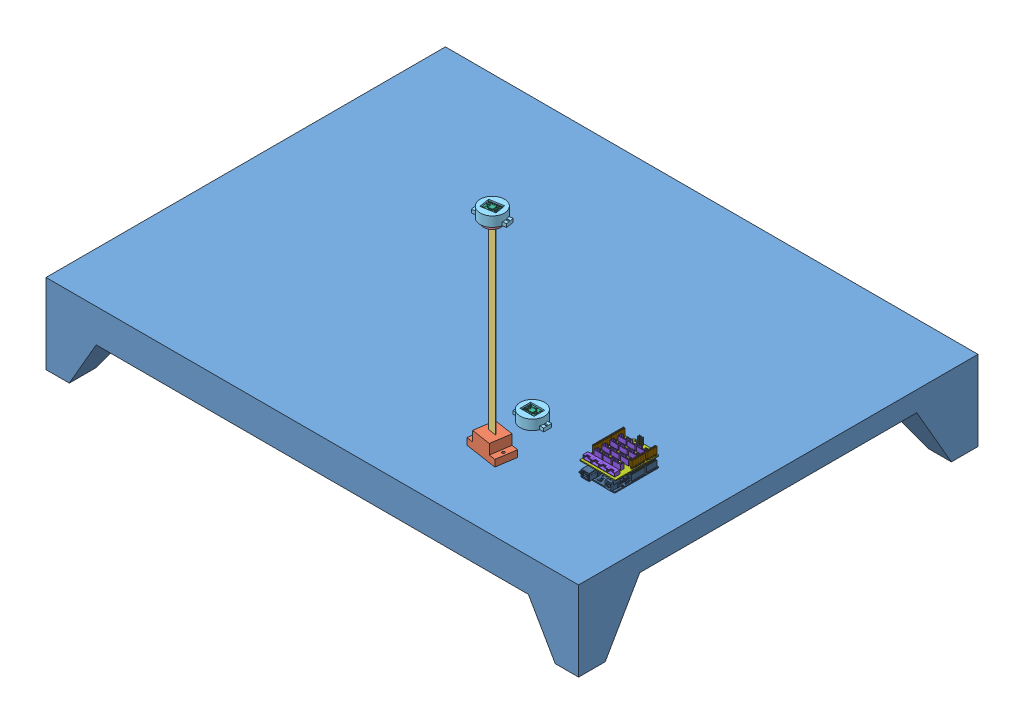
SolidWorks assembly ensamble Total, configuration Predeterminado. Lengths in mm.
Overall size (800 439 600).
75 component instances, 10 part files, 3 mates.
Components (placement in the parent):
- Mesa-1: Mesa [Predeterminado] at origin size (800 120 600)
- Edificio-1: Edificio [Predeterminado] at (161.3756 72.5 190.9633) x (0.988695 0 0.149939) z (-0.149939 0 0.988695) size (55.04 319 48.82)
  - baseSegueta-1: baseSegueta [Predeterminado] at origin size (50 25 30)
  - segueta-1: segueta [Predeterminado] at (0 142.5 0) size (12 310 0.8)
  - capuchon-1: capuchon [Predeterminado] at (3.1645 288.8301 -25.4) size (55.04 51.55 48.82)
    - masa-1: masa [Predeterminado] at (-3.1645 2.4199 25.4) size (25.4 12.5 25.4)
    - capuchon-1: capuchon [Predeterminado] at (-3.1645 8.6699 25.4) x (-0.949355 0 0.314206) z (-0.314206 0 -0.949355) size (46 51.55 36.2)
    - MPU6050 v2.step-1: MPU6050 v2.step [Predeterminado] at (-10.3102 15.6699 35.9917) x (0.314206 0 0.949355) z (-0.949355 0 0.314206) size (15.56 2 20.26)
- Microcontrolador-1: Microcontrolador [Predeterminado] at (314.2122 67.9538 160.0774) size (53.48 30.58 75.74)
  - Base Shield-1: Base Shield [Défaut] at (-27.6351 -53.574 -33.8465) x (0 0 -1) z (0 1 0) size (68.53 53.3 23.9)
    - Plaque support BSG-1: Plaque support BSG [Défaut] at (1.2775 -1.1272 67.25) size (68.53 53.3 1.5)
    - Grove Connecteur BSG-1: Grove Connecteur BSG [Défaut] at (18.4925 14.5228 78) x (0 0 -1) z (0 -1 0) size (7.8 5.3 12)
    - Grove Connecteur BSG-2: Grove Connecteur BSG [Défaut] at (18.4925 0.5228 78) x (0 0 -1) z (0 -1 0) size (7.8 5.3 12)
    - Grove Connecteur BSG-3: Grove Connecteur BSG [Défaut] at (18.4925 -13.4772 78) x (0 0 -1) z (0 -1 0) size (7.8 5.3 12)
    - Grove Connecteur BSG-4: Grove Connecteur BSG [Défaut] at (6.4925 14.5228 78) x (0 0 -1) z (0 -1 0) size (7.8 5.3 12)
    - Grove Connecteur BSG-5: Grove Connecteur BSG [Défaut] at (6.4925 0.5228 78) x (0 0 -1) z (0 -1 0) size (7.8 5.3 12)
    - Grove Connecteur BSG-6: Grove Connecteur BSG [Défaut] at (6.4925 -13.4772 78) x (0 0 -1) z (0 -1 0) size (7.8 5.3 12)
    - Grove Connecteur BSG-7: Grove Connecteur BSG [Défaut] at (-5.5075 14.5228 78) x (0 0 -1) z (0 -1 0) size (7.8 5.3 12)
    - Grove Connecteur BSG-8: Grove Connecteur BSG [Défaut] at (-5.5075 0.5228 78) x (0 0 -1) z (0 -1 0) size (7.8 5.3 12)
    - Grove Connecteur BSG-9: Grove Connecteur BSG [Défaut] at (-5.5075 -13.4772 78) x (0 0 -1) z (0 -1 0) size (7.8 5.3 12)
    - Grove Connecteur BSG-10: Grove Connecteur BSG [Défaut] at (-17.5075 14.5228 78) x (0 0 -1) z (0 -1 0) size (7.8 5.3 12)
    - Grove Connecteur BSG-11: Grove Connecteur BSG [Défaut] at (-17.5075 0.5228 78) x (0 0 -1) z (0 -1 0) size (7.8 5.3 12)
    - Grove Connecteur BSG-12: Grove Connecteur BSG [Défaut] at (-17.5075 -13.4772 78) x (0 0 -1) z (0 -1 0) size (7.8 5.3 12)
    - Grove Connecteur BSG-13: Grove Connecteur BSG [Défaut] at (-30.9375 18.5228 68) x (1 0 0) z (0 -1 0) size (7.8 5.3 12)
    - Grove Connecteur BSG-14: Grove Connecteur BSG [Défaut] at (-30.9375 6.5228 68) x (1 0 0) z (0 -1 0) size (7.8 5.3 12)
    - Grove Connecteur BSG-15: Grove Connecteur BSG [Défaut] at (-30.9375 -5.4772 68) x (1 0 0) z (0 -1 0) size (7.8 5.3 12)
    - Grove Connecteur BSG-16: Grove Connecteur BSG [Défaut] at (-30.9375 -17.4772 68) x (1 0 0) z (0 -1 0) size (7.8 5.3 12)
    - Barre_8pins_bs_bleu-1: Barre_8pins_bs_bleu [Défaut] at (5.8965 28.1355 69.3083) x (0 1 0) z (1 0 0) size (2.54 23.88 20.32)
      - Pin_bs_bleu-1: Pin_bs_bleu [Défaut] at (-5.3827 -0.5583 23.876) size (2.54 23.88 2.54)
      - Pin_bs_bleu-2: Pin_bs_bleu [Défaut] at (-5.3827 -0.5583 21.336) size (2.54 23.88 2.54)
      - Pin_bs_bleu-3: Pin_bs_bleu [Défaut] at (-5.3827 -0.5583 18.796) size (2.54 23.88 2.54)
      - Pin_bs_bleu-4: Pin_bs_bleu [Défaut] at (-5.3827 -0.5583 16.256) size (2.54 23.88 2.54)
      - Pin_bs_bleu-5: Pin_bs_bleu [Défaut] at (-5.3827 -0.5583 13.716) size (2.54 23.88 2.54)
      - Pin_bs_bleu-6: Pin_bs_bleu [Défaut] at (-5.3827 -0.5583 11.176) size (2.54 23.88 2.54)
      - Pin_bs_bleu-7: Pin_bs_bleu [Défaut] at (-5.3827 -0.5583 8.636) size (2.54 23.88 2.54)
      - Pin_bs_bleu-8: Pin_bs_bleu [Défaut] at (-5.3827 -0.5583 6.096) size (2.54 23.88 2.54)
    - Barre_8pins_bs_bleu-2: Barre_8pins_bs_bleu [Défaut] at (-11.3435 -19.6245 69.3083) x (0 1 0) z (1 0 0) size (2.54 23.88 20.32)
      - Pin_bs_bleu-1: Pin_bs_bleu [Défaut] at (-5.3827 -0.5583 23.876) size (2.54 23.88 2.54)
      - Pin_bs_bleu-2: Pin_bs_bleu [Défaut] at (-5.3827 -0.5583 21.336) size (2.54 23.88 2.54)
      - Pin_bs_bleu-3: Pin_bs_bleu [Défaut] at (-5.3827 -0.5583 18.796) size (2.54 23.88 2.54)
      - Pin_bs_bleu-4: Pin_bs_bleu [Défaut] at (-5.3827 -0.5583 16.256) size (2.54 23.88 2.54)
      - Pin_bs_bleu-5: Pin_bs_bleu [Défaut] at (-5.3827 -0.5583 13.716) size (2.54 23.88 2.54)
      - Pin_bs_bleu-6: Pin_bs_bleu [Défaut] at (-5.3827 -0.5583 11.176) size (2.54 23.88 2.54)
      - Pin_bs_bleu-7: Pin_bs_bleu [Défaut] at (-5.3827 -0.5583 8.636) size (2.54 23.88 2.54)
      - Pin_bs_bleu-8: Pin_bs_bleu [Défaut] at (-5.3827 -0.5583 6.096) size (2.54 23.88 2.54)
    - Barre_10pins_bs_bleu-1: Barre_10pins_bs_bleu [Défaut] at (-15.4235 28.6772 68.4619) x (0 1 0) z (1 0 0) size (2.54 23.88 25.4)
      - Pin_bs_bleu-1: Pin_bs_bleu [Défaut] at (-5.9244 0.2881 23.876) size (2.54 23.88 2.54)
      - Pin_bs_bleu-2: Pin_bs_bleu [Défaut] at (-5.9244 0.2881 21.336) size (2.54 23.88 2.54)
      - Pin_bs_bleu-3: Pin_bs_bleu [Défaut] at (-5.9244 0.2881 18.796) size (2.54 23.88 2.54)
      - Pin_bs_bleu-4: Pin_bs_bleu [Défaut] at (-5.9244 0.2881 16.256) size (2.54 23.88 2.54)
      - Pin_bs_bleu-5: Pin_bs_bleu [Défaut] at (-5.9244 0.2881 13.716) size (2.54 23.88 2.54)
      - Pin_bs_bleu-6: Pin_bs_bleu [Défaut] at (-5.9244 0.2881 11.176) size (2.54 23.88 2.54)
      - Pin_bs_bleu-7: Pin_bs_bleu [Défaut] at (-5.9244 0.2881 8.636) size (2.54 23.88 2.54)
      - Pin_bs_bleu-8: Pin_bs_bleu [Défaut] at (-5.9244 0.2881 6.096) size (2.54 23.88 2.54)
      - Pin_bs_bleu-9: Pin_bs_bleu [Défaut] at (-5.9244 0.2881 3.556) size (2.54 23.88 2.54)
      - Pin_bs_bleu-10: Pin_bs_bleu [Défaut] at (-5.9244 0.2881 1.016) size (2.54 23.88 2.54)
    - Barre_6pins_bs_bleu-1: Barre_6pins_bs_bleu [Défaut] at (40.9485 -29.1712 69.6807) x (0 -1 0) z (-1 0 0) size (2.54 23.88 15.24)
      - Pin_bs_bleu-1: Pin_bs_bleu [Défaut] at (-4.164 -0.9307 23.876) size (2.54 23.88 2.54)
      - Pin_bs_bleu-2: Pin_bs_bleu [Défaut] at (-4.164 -0.9307 21.336) size (2.54 23.88 2.54)
      - Pin_bs_bleu-3: Pin_bs_bleu [Défaut] at (-4.164 -0.9307 18.796) size (2.54 23.88 2.54)
      - Pin_bs_bleu-4: Pin_bs_bleu [Défaut] at (-4.164 -0.9307 16.256) size (2.54 23.88 2.54)
      - Pin_bs_bleu-5: Pin_bs_bleu [Défaut] at (-4.164 -0.9307 13.716) size (2.54 23.88 2.54)
      - Pin_bs_bleu-6: Pin_bs_bleu [Défaut] at (-4.164 -0.9307 11.176) size (2.54 23.88 2.54)
    - Barre_2x3pins_bs_bleu-1: Barre_2x3pins_bs_bleu [Défaut] at (32.0268 25.4488 65.8454) x (-1 0 0) z (0 -1 0) size (5.08 23.88 7.62)
      - Pin_bs_bleu-1: Pin_bs_bleu [Défaut] at (1.7942 -1.4046 23.876) size (2.54 23.88 2.54)
      - Pin_bs_bleu-2: Pin_bs_bleu [Défaut] at (-0.7458 -1.4046 23.876) size (2.54 23.88 2.54)
      - Pin_bs_bleu-3: Pin_bs_bleu [Défaut] at (1.7942 -1.4046 26.416) size (2.54 23.88 2.54)
      - Pin_bs_bleu-4: Pin_bs_bleu [Défaut] at (-0.7458 -1.4046 26.416) size (2.54 23.88 2.54)
      - Pin_bs_bleu-5: Pin_bs_bleu [Défaut] at (1.7942 -1.4046 28.956) size (2.54 23.88 2.54)
      - Pin_bs_bleu-6: Pin_bs_bleu [Défaut] at (-0.7458 -1.4046 28.956) size (2.54 23.88 2.54)
  - Arduino Uno(1)-1: Arduino Uno(1) [Default] at origin size (53.34 15.25 74.93)
- Cable_1-ensamble Total-1: Cable_1-ensamble Total [Predeterminado] at origin
- capuchon sin masa-1: capuchon sin masa [Predeterminado] at (151.7904 66 121.1866) size (46 15 36.2)
  - capuchon-1: capuchon [Predeterminado] at origin size (46 51.55 36.2)
  - MPU6050 v2.step-1: MPU6050 v2.step [Predeterminado] at (10.1118 7 -7.81) x (0 0 -1) z (1 0 0) size (15.56 2 20.26)
Mates (geometry in assembly coordinates):
- Coincidente3: coordinate: point of Mesa-1
- Coincidente2: coincident anti-aligned: plane of Mesa-1 through (-400 60 300) normal (0 1 0); plane of Edificio-1/baseSegueta-1 through (159.1265 60 205.7937) normal (0 -1 0)
- Coincidente4: coincident anti-aligned: plane of Mesa-1 through (-400 60 300) normal (0 1 0); plane of capuchon sin masa-1/capuchon-1 through (133.6904 60 121.1866) normal (0 -1 0)
